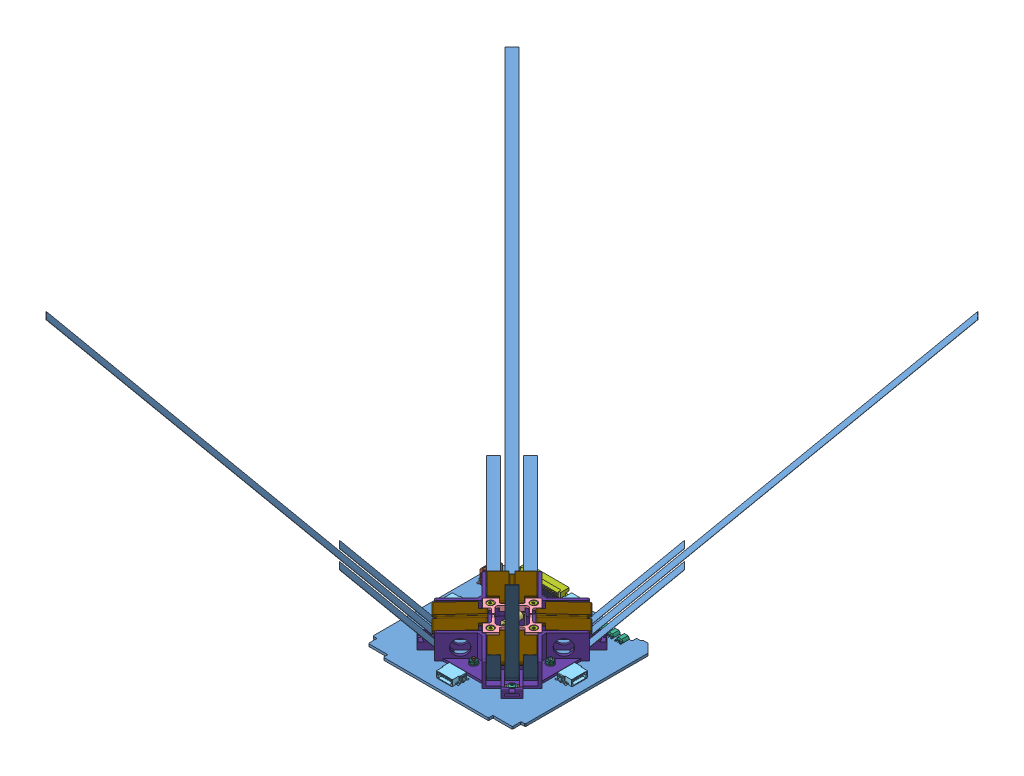
SolidWorks assembly 1U+Zendcard, configuration Deployed. Lengths in mm.
Overall size (309.73 193.28 309.73).
94 component instances, 25 part files, 155 mates.
Components (placement in the parent):
- 1UEndCardPCB-1: 1UEndCardPCB [Circular Turnstile] at origin
- m55-7011242_asm-2: m55-7011242_asm [Default] at (-42.5 0.8 -28.9) x (0 0 1) z (0 1 0) size (12.7 7.2 9)
  - m55-7011242_asm.stp-1: m55-7011242_asm.stp [Default] at origin size (12.7 7.2 9)
    - M55-70112_MOULD.stp-1: M55-70112_MOULD.stp [Default] at origin size (12.7 4.2 9)
    - M55-701_CONTACT.stp-1: M55-701_CONTACT.stp [Default] at (-3.175 -0.785 7.25) x (1 0 0) z (0 1 0) size (1.1 7.25 2.42)
    - M55-701_CONTACT.stp-2: M55-701_CONTACT.stp [Default] at (-1.905 -0.785 7.25) x (1 0 0) z (0 1 0) size (1.1 7.25 2.42)
    - M55-701_CONTACT.stp-3: M55-701_CONTACT.stp [Default] at (-0.635 -0.785 7.25) x (1 0 0) z (0 1 0) size (1.1 7.25 2.42)
    - M55-701_CONTACT.stp-4: M55-701_CONTACT.stp [Default] at (0.635 -0.785 7.25) x (1 0 0) z (0 1 0) size (1.1 7.25 2.42)
    - M55-701_CONTACT.stp-5: M55-701_CONTACT.stp [Default] at (1.905 -0.785 7.25) x (1 0 0) z (0 1 0) size (1.1 7.25 2.42)
    - M55-701_CONTACT.stp-6: M55-701_CONTACT.stp [Default] at (3.175 -0.785 7.25) x (1 0 0) z (0 1 0) size (1.1 7.25 2.42)
    - M55-701_CONTACT.stp-7: M55-701_CONTACT.stp [Default] at (-3.175 0.785 7.25) x (-1 0 0) z (0 -1 0) size (1.1 7.25 2.42)
    - M55-701_CONTACT.stp-8: M55-701_CONTACT.stp [Default] at (-1.905 0.785 7.25) x (-1 0 0) z (0 -1 0) size (1.1 7.25 2.42)
    - M55-701_CONTACT.stp-9: M55-701_CONTACT.stp [Default] at (-0.635 0.785 7.25) x (-1 0 0) z (0 -1 0) size (1.1 7.25 2.42)
    - M55-701_CONTACT.stp-10: M55-701_CONTACT.stp [Default] at (0.635 0.785 7.25) x (-1 0 0) z (0 -1 0) size (1.1 7.25 2.42)
    - M55-701_CONTACT.stp-11: M55-701_CONTACT.stp [Default] at (1.905 0.785 7.25) x (-1 0 0) z (0 -1 0) size (1.1 7.25 2.42)
    - M55-701_CONTACT.stp-12: M55-701_CONTACT.stp [Default] at (3.175 0.785 7.25) x (-1 0 0) z (0 -1 0) size (1.1 7.25 2.42)
    - M55-700_STRAP.stp-1: M55-700_STRAP.stp [Default] at (-5.67 0 0) x (1 0 0) z (0 -1 0) size (1 3.25 7.2)
    - M55-700_STRAP.stp-2: M55-700_STRAP.stp [Default] at (5.67 0 0) x (-1 0 0) z (0 1 0) size (1 3.25 7.2)
- m55-7101242_asm_defeature-1: m55-7101242_asm_defeature [Default] at (0 2.9 -35.35) x (-1 0 0) z (0 0 -1)
- m55-7101242_asm_defeature-2: m55-7101242_asm_defeature [Default] at (-35.35 2.9 0) x (0 0 1) z (-1 0 0)
- m55-7101242_asm_defeature-3: m55-7101242_asm_defeature [Default] at (35.35 2.9 0) x (0 0 -1) z (1 0 0)
- m55-7101242_asm_defeature-4: m55-7101242_asm_defeature [Default] at (0 2.9 35.35)
- Molex, LLC 0733000020 (Card Connector)-1: Molex, LLC 0733000020 (Card Connector) [Default] at (22.001 0.9778 -40.8) x (-1 0 0) z (0 0 -1)
- Molex, LLC 0733000020 (Card Connector)-2: Molex, LLC 0733000020 (Card Connector) [Default] at (28.001 0.9778 -40.8) x (-1 0 0) z (0 0 -1)
- Molex, LLC 0733000020 (Card Connector)-3: Molex, LLC 0733000020 (Card Connector) [Default] at (33.999 0.9778 -40.8) x (-1 0 0) z (0 0 -1)
- TFM_120_01_L_D_RA-1: TFM_120_01_L_D_RA [Default] at (-21.65 3.6575 -39.237) x (-1 0 0) z (0 -1 0) size (28.58 7.49 7.62)
  - _TFM_120_01_L_D_RA_terminal_2-1: _TFM_120_01_L_D_RA_terminal_2 [Default] at origin size (28.58 5.59 5.72)
  - _TFM_120_01_L_D_RA_pins_4-1: _TFM_120_01_L_D_RA_pins_4 [Default] at origin size (25.4 6.95 5.84)
- MezzaninePCB-1: MezzaninePCB [Default] at (0 -4.4 0) x (1 0 0) z (0 1 0)
- R107.064.070C-1: R107.064.070C [Default] at (23.4 -2.8 -23.4) x (0 1 0) z (0.707107 0 -0.707107)
- R107.064.070C-2: R107.064.070C [Default] at (38.1 -2.8 -26.1) x (0 1 0) z (1 0 0)
- R107.064.070C-5: R107.064.070C [Default] at (23.4 -2.8 23.4) x (0 1 0) z (0.707107 0 0.707107)
- R107.064.070C-6: R107.064.070C [Default] at (-23.4 -2.8 23.4) x (0 1 0) z (-0.707107 0 0.707107)
- R107.064.070C-7: R107.064.070C [Default] at (-23.4 -2.8 -23.4) x (0 1 0) z (-0.707107 0 -0.707107)
- 90265A113_18-8 STAINLESS STEEL SHOULDER SCREW-1: 90265A113_18-8 STAINLESS STEEL SHOULDER SCREW [90265A113] at (0 -6.4 -25.1) x (-1 0 0) z (0 -1 0)
- 90265A113_18-8 STAINLESS STEEL SHOULDER SCREW-2: 90265A113_18-8 STAINLESS STEEL SHOULDER SCREW [90265A113] at (0 -6.4 25.1) x (-0.982925 0 0.184007) z (0 -1 0)
- 94669A212_ALUM UNTHRD SPACER-1: 94669A212_ALUM UNTHRD SPACER [94669A212] at (0 -1.8 -25.1) x (-0.837169 0 -0.546944) z (0 1 0)
- 94669A212_ALUM UNTHRD SPACER-2: 94669A212_ALUM UNTHRD SPACER [94669A212] at (0 -1.8 25.1) x (0.982925 0 -0.184007) z (0 1 0)
- 94669A211_ALUM UNTHRD SPACER-3: 94669A211_ALUM UNTHRD SPACER [94669A211] at (25.1 -1.8 0) x (1 0 0) z (0 -1 0)
- 94669A211_ALUM UNTHRD SPACER-4: 94669A211_ALUM UNTHRD SPACER [94669A211] at (-25.1 -1.8 0) x (1 0 0) z (0 -1 0)
- 92855A840_18-8 SS LOW-PROFILE SCKT HEAD SCREWS-1: 92855A840_18-8 SS LOW-PROFILE SCKT HEAD SCREWS [92855A840] at (-25.1 5.6 0) x (1 0 0) z (0 1 0)
- 92855A840_18-8 SS LOW-PROFILE SCKT HEAD SCREWS-2: 92855A840_18-8 SS LOW-PROFILE SCKT HEAD SCREWS [92855A840] at (25.1 5.6 0) x (1 0 0) z (0 1 0)
- 91828A111_TYPE 18-8 STAINLESS STEEL HEX NUT-4: 91828A111_TYPE 18-8 STAINLESS STEEL HEX NUT [91828A111] at (-25.1 3.5 0) x (0.837169 0 0.546944) z (0 -1 0)
- 94100A150_18-8 SS PRESS-FIT NUT FOR SOFT MTL PLASTIC-1: 94100A150_18-8 SS PRESS-FIT NUT FOR SOFT MTL PLASTIC [94100A150] at (27.0307 -2.3 27.0307) x (1 0 0) z (0 -1 0)
- 94100A150_18-8 SS PRESS-FIT NUT FOR SOFT MTL PLASTIC-2: 94100A150_18-8 SS PRESS-FIT NUT FOR SOFT MTL PLASTIC [94100A150] at (-27.0307 -2.3 27.0307) x (0 0 1) z (0 -1 0)
- 94100A150_18-8 SS PRESS-FIT NUT FOR SOFT MTL PLASTIC-3: 94100A150_18-8 SS PRESS-FIT NUT FOR SOFT MTL PLASTIC [94100A150] at (-27.0307 -2.3 -27.0307) x (-1 0 0) z (0 -1 0)
- 94100A150_18-8 SS PRESS-FIT NUT FOR SOFT MTL PLASTIC-4: 94100A150_18-8 SS PRESS-FIT NUT FOR SOFT MTL PLASTIC [94100A150] at (27.0307 -2.3 -27.0307) x (0 0 -1) z (0 -1 0)
- TapeMeasureMount-1: TapeMeasureMount [Vented Fastener melt wire] at (0 0.3 0) size (70.66 21.28 70.66)
- Trapdoor-2: Trapdoor [Default] at (-17.0117 16.4693 17.0117) x (-0.707107 0 -0.707107) z (-0.706844 -0.027263 0.706844) size (23 3.2 26)
- TurnstyleElements-1: TurnstyleElements [L band] at (-12.6549 0.8 29.2719) x (-0.707107 0 0.707107) z (-0.707107 0 -0.707107)
- TurnstyleElements-2: TurnstyleElements [L band] at (-24.6757 0.8 17.2511) x (-0.707107 0 0.707107) z (-0.707107 0 -0.707107)
- TurnstyleElements-3: TurnstyleElements [UHF band] at (-18.6653 0.8 23.2615) x (-0.707107 0 0.707107) z (-0.707107 0 -0.707107)
- squarewasher-1: squarewasher [Default] at (-27.3735 2.65 27.3735) x (0.707107 0 0.707107) z (-0.707107 0 0.707107) size (6.5 0.75 5)
- PAC01_VIS-1: PAC01_VIS [Taller Soldering (1U Endcard)] at (0 12.094 8.75) x (0 0 -1) z (0 1 0) size (18.41 4.29 15.59)
- topCap-1: topCap [Default] at (-11.3137 15.4 -0.1414) x (0.707107 0 0.707107) z (-0.707107 0 0.707107) size (27.5 3.5 27.5)
- TurnstyleElements-13: TurnstyleElements [L band] at (-17.2511 0.8 -24.6757) x (-0.707107 0 -0.707107) z (0.707107 0 -0.707107)
- TurnstyleElements-14: TurnstyleElements [L band] at (24.6757 0.8 -17.2511) x (0.707107 0 -0.707107) z (0.707107 0 0.707107)
- TurnstyleElements-15: TurnstyleElements [L band] at (17.2511 0.8 24.6757) x (0.707107 0 0.707107) z (-0.707107 0 0.707107)
- TurnstyleElements-16: TurnstyleElements [UHF band] at (-23.2615 0.8 -18.6653) x (-0.707107 0 -0.707107) z (0.707107 0 -0.707107)
- TurnstyleElements-17: TurnstyleElements [UHF band] at (18.6653 0.8 -23.2615) x (0.707107 0 -0.707107) z (0.707107 0 0.707107)
- TurnstyleElements-18: TurnstyleElements [UHF band] at (23.2615 0.8 18.6653) x (0.707107 0 0.707107) z (-0.707107 0 0.707107)
- TurnstyleElements-19: TurnstyleElements [L band] at (-29.2719 0.8 -12.6549) x (-0.707107 0 -0.707107) z (0.707107 0 -0.707107)
- TurnstyleElements-20: TurnstyleElements [L band] at (12.6549 0.8 -29.2719) x (0.707107 0 -0.707107) z (0.707107 0 0.707107)
- TurnstyleElements-21: TurnstyleElements [L band] at (29.2719 0.8 12.6549) x (0.707107 0 0.707107) z (-0.707107 0 0.707107)
- squarewasher-5: squarewasher [Default] at (-27.3735 2.65 -27.3735) x (-0.707107 0 0.707107) z (-0.707107 0 -0.707107) size (6.5 0.75 5)
- squarewasher-6: squarewasher [Default] at (27.3735 2.65 -27.3735) x (-0.707107 0 -0.707107) z (0.707107 0 -0.707107) size (6.5 0.75 5)
- squarewasher-7: squarewasher [Default] at (27.3735 2.65 27.3735) x (0.707107 0 -0.707107) z (0.707107 0 0.707107) size (6.5 0.75 5)
- Trapdoor-6: Trapdoor [Default] at (-17.0117 16.4693 -17.0117) x (0.707107 0 -0.707107) z (-0.706844 -0.027263 -0.706844) size (23 3.2 26)
- Trapdoor-7: Trapdoor [Default] at (17.0117 16.4693 -17.0117) x (0.707107 0 0.707107) z (0.706844 -0.027263 -0.706844) size (23 3.2 26)
- Trapdoor-8: Trapdoor [Default] at (17.0117 16.4693 17.0117) x (-0.707107 0 0.707107) z (0.706844 -0.027263 0.706844) size (23 3.2 26)
- 94100A150_18-8 SS PRESS-FIT NUT FOR SOFT MTL PLASTIC-5: 94100A150_18-8 SS PRESS-FIT NUT FOR SOFT MTL PLASTIC [94100A150] at (-27.0307 -2.3 -27.0307) x (-1 0 0) z (0 -1 0)
- 90965A110_TYPE 316 STAINLESS STEEL FLAT WASHER-1: 90965A110_TYPE 316 STAINLESS STEEL FLAT WASHER [90965A110] at (-27.0307 3.4 27.0307) x (0 0 -1) z (0 1 0) size (5 5 0.4)
- 90910A922_LOW-PROFILE BUTTON HEAD TORX MACHINE SCREW-1: 90910A922_LOW-PROFILE BUTTON HEAD TORX MACHINE SCREW [90910A922] at (-27.0307 4.9 27.0307) x (1 0 0) z (0 1 0) size (3.8 3.8 7.25)
- 90910A922_LOW-PROFILE BUTTON HEAD TORX MACHINE SCREW-2: 90910A922_LOW-PROFILE BUTTON HEAD TORX MACHINE SCREW [90910A922] at (-27.0307 4.9 -27.0307) x (0 0 1) z (0 1 0) size (3.8 3.8 7.25)
- 90910A922_LOW-PROFILE BUTTON HEAD TORX MACHINE SCREW-3: 90910A922_LOW-PROFILE BUTTON HEAD TORX MACHINE SCREW [90910A922] at (27.0307 4.9 -27.0307) x (-1 0 0) z (0 1 0) size (3.8 3.8 7.25)
- 90910A922_LOW-PROFILE BUTTON HEAD TORX MACHINE SCREW-4: 90910A922_LOW-PROFILE BUTTON HEAD TORX MACHINE SCREW [90910A922] at (27.0307 4.9 27.0307) x (0 0 -1) z (0 1 0) size (3.8 3.8 7.25)
- 90965A110_TYPE 316 STAINLESS STEEL FLAT WASHER-2: 90965A110_TYPE 316 STAINLESS STEEL FLAT WASHER [90965A110] at (-27.0307 3.4 -27.0307) x (1 0 0) z (0 1 0) size (5 5 0.4)
- 90965A110_TYPE 316 STAINLESS STEEL FLAT WASHER-3: 90965A110_TYPE 316 STAINLESS STEEL FLAT WASHER [90965A110] at (27.0307 3.4 -27.0307) x (0 0 1) z (0 1 0) size (5 5 0.4)
- 90965A110_TYPE 316 STAINLESS STEEL FLAT WASHER-4: 90965A110_TYPE 316 STAINLESS STEEL FLAT WASHER [90965A110] at (27.0307 3.4 27.0307) x (-1 0 0) z (0 1 0) size (5 5 0.4)
- 91828A111_TYPE 18-8 STAINLESS STEEL HEX NUT-5: 91828A111_TYPE 18-8 STAINLESS STEEL HEX NUT [91828A111] at (14.1421 12.5 0) x (0.965926 0 -0.258819) z (0 1 0)
- 91828A111_TYPE 18-8 STAINLESS STEEL HEX NUT-6: 91828A111_TYPE 18-8 STAINLESS STEEL HEX NUT [91828A111] at (-14.1421 12.5 0) x (-0.965926 0 0.258819) z (0 1 0)
- 91828A111_TYPE 18-8 STAINLESS STEEL HEX NUT-7: 91828A111_TYPE 18-8 STAINLESS STEEL HEX NUT [91828A111] at (0 12.5 14.1421) x (0.965926 0 -0.258819) z (0 1 0)
- 91828A111_TYPE 18-8 STAINLESS STEEL HEX NUT-8: 91828A111_TYPE 18-8 STAINLESS STEEL HEX NUT [91828A111] at (0 12.5 -14.1421) x (-0.965926 0 0.258819) z (0 1 0)
- 92703A145_18-8 STAINLESS STEEL TORX FLAT HEAD SCREWS (1)-1: 92703A145_18-8 STAINLESS STEEL TORX FLAT HEAD SCREWS (1) [92703A145] at (14.1421 16.75 -0.1414) x (1 0 0) z (0 1 0) size (3.78 3.78 6.2)
- 92703A145_18-8 STAINLESS STEEL TORX FLAT HEAD SCREWS (1)-2: 92703A145_18-8 STAINLESS STEEL TORX FLAT HEAD SCREWS (1) [92703A145] at (0.1414 16.75 14.1421) x (0 0 1) z (0 1 0) size (3.78 3.78 6.2)
- 92703A145_18-8 STAINLESS STEEL TORX FLAT HEAD SCREWS (1)-3: 92703A145_18-8 STAINLESS STEEL TORX FLAT HEAD SCREWS (1) [92703A145] at (-14.1421 16.75 0.1414) x (-1 0 0) z (0 1 0) size (3.78 3.78 6.2)
- 92703A145_18-8 STAINLESS STEEL TORX FLAT HEAD SCREWS (1)-4: 92703A145_18-8 STAINLESS STEEL TORX FLAT HEAD SCREWS (1) [92703A145] at (-0.1414 16.75 -14.1421) x (0 0 -1) z (0 1 0) size (3.78 3.78 6.2)
- 91828A111_TYPE 18-8 STAINLESS STEEL HEX NUT-9: 91828A111_TYPE 18-8 STAINLESS STEEL HEX NUT [91828A111] at (0 3.5 -25.1) x (-0.546944 0 0.837169) z (0 -1 0)
- 91828A111_TYPE 18-8 STAINLESS STEEL HEX NUT-10: 91828A111_TYPE 18-8 STAINLESS STEEL HEX NUT [91828A111] at (25.1 3.5 0) x (-0.837169 0 -0.546944) z (0 -1 0)
- 91828A111_TYPE 18-8 STAINLESS STEEL HEX NUT-11: 91828A111_TYPE 18-8 STAINLESS STEEL HEX NUT [91828A111] at (0 3.5 25.1) x (0.546944 0 -0.837169) z (0 -1 0)
- 90965A110_TYPE 316 STAINLESS STEEL FLAT WASHER-5: 90965A110_TYPE 316 STAINLESS STEEL FLAT WASHER [90965A110] at (-25.1 2.7 0) x (0.546944 0 -0.837169) z (0 -1 0) size (5 5 0.4)
- 90965A110_TYPE 316 STAINLESS STEEL FLAT WASHER-6: 90965A110_TYPE 316 STAINLESS STEEL FLAT WASHER [90965A110] at (0 2.7 -25.1) x (0.837169 0 0.546944) z (0 -1 0) size (5 5 0.4)
- 90965A110_TYPE 316 STAINLESS STEEL FLAT WASHER-7: 90965A110_TYPE 316 STAINLESS STEEL FLAT WASHER [90965A110] at (25.1 2.7 0) x (-0.546944 0 0.837169) z (0 -1 0) size (5 5 0.4)
- 90965A110_TYPE 316 STAINLESS STEEL FLAT WASHER-8: 90965A110_TYPE 316 STAINLESS STEEL FLAT WASHER [90965A110] at (0 2.7 25.1) x (-0.837169 0 -0.546944) z (0 -1 0) size (5 5 0.4)
Mates (geometry in assembly coordinates):
- Parallel2: parallel aligned: plane of 1UEndCardPCB-1 through (-49.9 -0.8 0) normal (-1 0 0); plane of m55-7011242_asm-2/m55-7011242_asm.stp-1/M55-70112_MOULD.stp-1 through (-44.6 0.8 -34.57) normal (-1 0 0)
- Concentric1: concentric anti-aligned: cylinder of 1UEndCardPCB-1 through (-42.5 -9.2 -34.285) axis (0 1 0) radius 0.8; circle of m55-7011242_asm-2/m55-7011242_asm.stp-1/M55-70112_MOULD.stp-1
- Coincident2: coincident anti-aligned: plane of 1UEndCardPCB-1 through (0 0.8 0) normal (0 1 0); plane of m55-7011242_asm-2/m55-7011242_asm.stp-1/M55-700_STRAP.stp-1 through (-42.5 0.8 -34.57) normal (0 -1 0)
- Concentric2: concentric aligned: circle of m55-7101242_asm_defeature-1; cylinder of 1UEndCardPCB-1 through (5.385 -0.8 -37.75) axis (0 1 0) radius 0.8
- Coincident3: coincident anti-aligned: plane of 1UEndCardPCB-1 through (0 0.8 0) normal (0 1 0); plane of m55-7101242_asm_defeature-1 through (5.67 0.8 -35.35) normal (0 -1 0)
- Parallel3: parallel aligned: plane of 1UEndCardPCB-1 through (0 -0.8 -44.8) normal (0 0 -1); plane of m55-7101242_asm_defeature-1 through (0 2.9 -44.15) normal (0 0 -1)
- Coincident4: coincident anti-aligned: plane of 1UEndCardPCB-1 through (0 0.8 0) normal (0 1 0); plane of m55-7101242_asm_defeature-2 through (-35.35 0.8 -5.67) normal (0 -1 0)
- Concentric4: concentric anti-aligned: circle of m55-7101242_asm_defeature-2; cylinder of 1UEndCardPCB-1 through (-37.75 -0.8 -5.385) axis (0 1 0) radius 0.8
- Parallel4: parallel aligned: plane of 1UEndCardPCB-1 through (-49.9 -0.8 0) normal (-1 0 0); plane of m55-7101242_asm_defeature-2 through (-44.15 2.9 0) normal (-1 0 0)
- Coincident6: coincident anti-aligned: plane of 1UEndCardPCB-1 through (0 0.8 0) normal (0 1 0); plane of m55-7101242_asm_defeature-4 through (-5.67 0.8 35.35) normal (0 -1 0)
- Concentric6: concentric anti-aligned: circle of m55-7101242_asm_defeature-4; cylinder of 1UEndCardPCB-1 through (-5.385 -0.8 37.75) axis (0 1 0) radius 0.8
- Parallel5: parallel aligned: plane of m55-7101242_asm_defeature-4 through (0 2.9 44.15) normal (0 0 1); plane of 1UEndCardPCB-1 through (34.4 -0.801 49.8) normal (0 0 1)
- Concentric7: concentric aligned: circle of m55-7101242_asm_defeature-3; cylinder of 1UEndCardPCB-1 through (37.75 -0.8 5.385) axis (0 1 0) radius 0.8
- Coincident7: coincident anti-aligned: plane of 1UEndCardPCB-1 through (0 0.8 0) normal (0 1 0); plane of m55-7101242_asm_defeature-3 through (35.35 0.8 5.67) normal (0 -1 0)
- Parallel6: parallel aligned: plane of 1UEndCardPCB-1 through (49.9 -0.8 0) normal (1 0 0); plane of m55-7101242_asm_defeature-3 through (44.15 2.9 0) normal (1 0 0)
- Coincident18: coincident anti-aligned: plane of 1UEndCardPCB-1 through (0 0.8 0) normal (0 1 0); plane of TFM_120_01_L_D_RA-1/_TFM_120_01_L_D_RA_terminal_2-1 through (-7.3625 0.8 -44.825) normal (0 -1 0)
- Coincident19: coincident: line of 1UEndCardPCB-1 through (-33.8928 0.8 -37.332) axis (0 0 -1); plane of TFM_120_01_L_D_RA-1/_TFM_120_01_L_D_RA_pins_4-1 through (-33.8928 -1.105 -39.999) normal (-1 0 0)
- Coincident20: coincident: line of 1UEndCardPCB-1 through (-9.4072 0.8 -37.332) axis (-1 0 0); plane of TFM_120_01_L_D_RA-1/_TFM_120_01_L_D_RA_pins_4-1 through (-21.65 3.6575 -37.332) normal (0 0 1)
- Coincident22: coincident anti-aligned: plane of 1UEndCardPCB-1 through (0 0.8 0) normal (0 1 0); plane of Molex, LLC 0733000020 (Card Connector)-3 through (33.999 0.8 -35.1866) normal (0 -1 0)
- Coincident23: coincident aligned: plane of 1UEndCardPCB-1 through (0 -0.8 -40.8) normal (0 0 -1); plane of Molex, LLC 0733000020 (Card Connector)-3 through (33.999 -0.6097 -40.8) normal (0 0 -1)
- Distance4: distance = 0.065 mm anti-aligned: plane of Molex, LLC 0733000020 (Card Connector)-3 through (32.475 0.8 -40.8) normal (-1 0 0); plane of 1UEndCardPCB-1 through (32.41 -0.8 0) normal (1 0 0)
- Coincident24: coincident anti-aligned: plane of 1UEndCardPCB-1 through (0 0.8 0) normal (0 1 0); plane of Molex, LLC 0733000020 (Card Connector)-2 through (28.001 0.8 -35.1866) normal (0 -1 0)
- Distance5: distance = 0.065 mm anti-aligned: plane of 1UEndCardPCB-1 through (29.59 -0.8 0) normal (-1 0 0); plane of Molex, LLC 0733000020 (Card Connector)-2 through (29.525 -0.6097 -40.8) normal (1 0 0)
- Coincident25: coincident aligned: plane of 1UEndCardPCB-1 through (0 -0.8 -40.8) normal (0 0 -1); plane of Molex, LLC 0733000020 (Card Connector)-2 through (28.001 -0.6097 -40.8) normal (0 0 -1)
- Coincident26: coincident anti-aligned: plane of 1UEndCardPCB-1 through (0 0.8 0) normal (0 1 0); plane of Molex, LLC 0733000020 (Card Connector)-1 through (22.001 0.8 -35.1866) normal (0 -1 0)
- Distance6: distance = 0.065 mm anti-aligned: plane of Molex, LLC 0733000020 (Card Connector)-1 through (23.525 -0.6097 -40.8) normal (1 0 0); plane of 1UEndCardPCB-1 through (23.59 -0.8 0) normal (-1 0 0)
- Coincident27: coincident aligned: plane of 1UEndCardPCB-1 through (0 -0.8 -40.8) normal (0 0 -1); plane of Molex, LLC 0733000020 (Card Connector)-1 through (22.001 -0.6097 -40.8) normal (0 0 -1)
- Coincident64: coincident anti-aligned: plane of 1UEndCardPCB-1 through (0 -0.8 0) normal (0 -1 0); plane of tunacan-1 through (5.1664 1.6055 -5.6105) normal (0 1 0)
- Concentric9: concentric aligned: circle of EndCardPCB-1; circle of tunacan-1
- Coincident65: coincident: line of 1UEndCardPCB-1 through (0 0.8 5.2282) axis (0 0 -1); plane of tunacan-1 through (5.1664 -24.6445 -5.6105) normal (1 0 0)
- Coincident70: coincident anti-aligned: plane of 1UEndCardPCB-1 through (0 -0.8 0) normal (0 -1 0); plane of halfinTurnstileMount-12 through (-25.9822 1.6055 27.1766) normal (0 1 0)
- Coincident72: coincident aligned: plane of halfinTurnstileMount-12 through (-25.9822 1.6055 27.1766) normal (0 0 -1); plane of Turnstile_Antenna-4 through (-153.4531 -161.0492 27.1766) normal (0 0 -1)
- Parallel22: parallel aligned: cylinder of halfinTurnstileMount-12 through (-5.5264 -13.1224 27.1766) axis (-0.707107 -0.707107 0) radius 25; cylinder of Turnstile_Antenna-4 through (-11.8904 -19.4864 27.1766) axis (-0.707107 -0.707107 0) radius 25
- Concentric11: concentric aligned: cylinder of halfinTurnstileMount-12 through (-5.5264 -13.1224 27.1766) axis (-0.707107 -0.707107 0) radius 25; cylinder of Turnstile_Antenna-4 through (-11.8904 -19.4864 27.1766) axis (-0.707107 -0.707107 0) radius 25
- Coincident73: coincident anti-aligned: plane of 1UEndCardPCB-1 through (0 -0.8 0) normal (0 -1 0); plane of halfinTurnstileMount-13 through (-27.6207 1.6055 -30.4458) normal (0 1 0)
- Coincident74: coincident anti-aligned: plane of 1UEndCardPCB-1 through (0 -0.8 0) normal (0 -1 0); plane of halfinTurnstileMount-11 through (30.0017 1.6055 -32.0842) normal (0 1 0)
- Coincident80: coincident anti-aligned: plane of Turnstile_Antenna-1 through (15.9098 -19.4864 -32.0842) normal (0 0 -1); plane of halfinTurnstileMount-11 through (30.0017 1.6055 -32.0842) normal (0 0 1)
- Tangent1: tangent aligned: cylinder of Turnstile_Antenna-1 through (157.4726 -161.0492 -32.0842) axis (-0.707107 0.707107 0) radius 25; cylinder of halfinTurnstileMount-11 through (9.5459 -13.1224 -32.0842) axis (0.707107 -0.707107 0) radius 25
- Coincident81: coincident anti-aligned: plane of 1UEndCardPCB-1 through (0 -0.8 0) normal (0 -1 0); plane of halfinTurnstileMount-14 through (31.6402 1.6055 25.5382) normal (0 1 0)
- Coincident82: coincident aligned: plane of halfinTurnstileMount-14 through (31.6402 1.6055 25.5382) normal (-1 0 0); plane of Turnstile_Antenna-3 through (31.6402 -161.0492 153.0091) normal (-1 0 0)
- Tangent2: tangent aligned: cylinder of halfinTurnstileMount-14 through (31.6402 -13.1224 5.0823) axis (0 -0.707107 0.707107) radius 25; cylinder of Turnstile_Antenna-3 through (31.6402 -19.4864 11.4463) axis (0 -0.707107 0.707107) radius 25
- Tangent3: tangent aligned: cylinder of halfinTurnstileMount-13 through (-27.6207 -13.1224 -9.9899) axis (0 -0.707107 -0.707107) radius 25; cylinder of Turnstile_Antenna-2 through (-27.6207 -19.4864 -16.3539) axis (0 -0.707107 -0.707107) radius 25
- Coincident92: coincident anti-aligned: circle of tunacan-1; plane of HARP-9002-A-2/HARP-9002-A.stp-1/navitar-solid-model_swir-25.stp-1 through (5.1664 -50.8945 -14.8605) normal (0 -1 0)
- Concentric12: concentric aligned: circle of tunacan-1; circle of HARP-9002-A-2/HARP-9002-A.stp-1/navitar-solid-model_swir-25.stp-1
- Parallel27: parallel aligned: plane of 1UEndCardPCB-1 through (0 -0.8 49.9) normal (0 0 1); plane of HARP-9002-A-2/HARP-9002-A.stp-1/instrument_electronics.stp-1/TIM PCB.stp-1 through (-41.2572 22.5257 42.352) normal (0 0 1)
- Coincident93: coincident aligned: plane of halfinTurnstileMount-13 through (-27.6207 1.6055 -30.4458) normal (1 0 0); plane of Turnstile_Antenna-2 through (-27.6207 -161.0492 -157.9167) normal (1 0 0)
- Tangent4: tangent aligned: cylinder of halfinTurnstileMount-13 through (-27.6207 -13.1224 -9.9899) axis (0 -0.707107 -0.707107) radius 25; cylinder of Turnstile_Antenna-2 through (-27.6207 -19.4864 -16.3539) axis (0 -0.707107 -0.707107) radius 25
- Parallel28: parallel aligned: cylinder of halfinTurnstileMount-13 through (-27.6207 -13.1224 -9.9899) axis (0 -0.707107 -0.707107) radius 25; cylinder of Turnstile_Antenna-2 through (-27.6207 -19.4864 -16.3539) axis (0 -0.707107 -0.707107) radius 25
- Coincident94: coincident anti-aligned: plane of halfinTurnstileMount-12 through (-29.4822 -1.8945 27.1766) normal (-0.707107 -0.707107 0); plane of Turnstile_Antenna-4 through (-11.8904 -19.4864 27.1766) normal (0.707107 0.707107 0)
- Coincident95: coincident anti-aligned: plane of halfinTurnstileMount-13 through (-27.6207 -1.8945 -33.9458) normal (0 -0.707107 -0.707107); plane of Turnstile_Antenna-2 through (-27.6207 -19.4864 -16.3539) normal (0 0.707107 0.707107)
- Coincident96: coincident anti-aligned: plane of Turnstile_Antenna-1 through (15.9098 -19.4864 -32.0842) normal (-0.707107 0.707107 0); plane of halfinTurnstileMount-11 through (33.5017 -1.8945 -32.0842) normal (0.707107 -0.707107 0)
- Coincident97: coincident anti-aligned: plane of halfinTurnstileMount-14 through (31.6402 -1.8945 29.0382) normal (0 -0.707107 0.707107); plane of Turnstile_Antenna-3 through (31.6402 -19.4864 11.4463) normal (0 0.707107 -0.707107)
- Coincident99: coincident: plane of halfinTurnstileMount-9; point of tunacan-1
- Coincident100: coincident anti-aligned: plane of halfinTurnstileMount-10; plane of halfinTurnstileMount-9
- Coincident101: coincident aligned: line of halfinTurnstileMount-11 through (40.353 -0.3945 -21.7864) axis (0 0 -1); line of halfinTurnstileMount-9 through (43.3496 -0.3945 21.665) axis (0 0 -1)
- Coincident103: coincident anti-aligned: plane of halfinTurnstileMount-6; plane of halfinTurnstileMount-11
- Coincident104: coincident aligned: line of halfinTurnstileMount-6 through (-19.1125 -0.3945 29.5761) axis (1 0 0); line of halfinTurnstileMount-9 through (24.3389 -0.3945 32.5726) axis (1 0 0)
- Coincident106: coincident: line of EndCardPCB-1 through (-30.0202 1.6055 -40.7971) axis (0 0 1); plane of halfinTurnstileMount-10 through (-30.0202 37.1592 -40.7971) normal (-1 0 0)
- Coincident108: coincident: line of EndCardPCB-1 through (-30.0202 1.6055 -40.7971) axis (0 0 1); plane of halfinTurnstileMount-6 through (-30.0202 37.1592 29.5761) normal (-1 0 0)
- Coincident109: coincident: line of EndCardPCB-1 through (-30.0202 1.6055 29.5761) axis (1 0 0); plane of halfinTurnstileMount-6 through (-30.0202 37.1592 29.5761) normal (0 0 1)
- Coincident121: coincident anti-aligned: plane of halfinTurnstileMount-12 through (-17.1447 4.6055 35.8895) normal (0 0 1); line of 1UEndCardPCB-1 through (-41.5 -0.8 41.5) axis (1 0 0)
- Coincident122: coincident: line of 1UEndCardPCB-1 through (-41.5 0.8 46.9) axis (0 0 -1); plane of halfinTurnstileMount-12 through (-36.3336 4.6055 35.8895) normal (-1 0 0)
- Coincident123: coincident: line of 1UEndCardPCB-1 through (-41.5 0.8 46.9) axis (0 0 -1); plane of halfinTurnstileMount-13 through (-36.3336 4.6055 -21.6083) normal (-1 0 0)
- Coincident124: coincident: line of 1UEndCardPCB-1 through (-35.1866 -0.8 -35.1866) axis (1 0 0); plane of halfinTurnstileMount-13 through (-36.3336 4.6055 -40.7971) normal (0 0 -1)
- Coincident125: coincident: line of 1UEndCardPCB-1 through (-35.1866 -0.8 -35.1866) axis (1 0 0); plane of halfinTurnstileMount-11 through (21.1642 4.6055 -40.7971) normal (0 0 -1)
- Coincident126: coincident: line of 1UEndCardPCB-1 through (35.1866 -0.8 -35.1866) axis (0 0 1); plane of halfinTurnstileMount-11 through (40.353 4.6055 -40.7971) normal (1 0 0)
- Coincident127: coincident aligned: line of 1UEndCardPCB-1 through (-41.5 -0.8 41.5) axis (1 0 0); plane of halfinTurnstileMount-14 through (40.353 4.6055 35.8895) normal (0 0 1)
- Coincident128: coincident: line of 1UEndCardPCB-1 through (35.1866 -0.8 -35.1866) axis (0 0 1); plane of halfinTurnstileMount-14 through (40.353 4.6055 16.7007) normal (1 0 0)
- Coincident129: coincident anti-aligned: plane of 1UEndCardPCB-1 through (0 -0.8 0) normal (0 -1 0); plane of Turnstile Mount-1 through (32.503 1.6055 18.8895) normal (0 1 0)
- Coincident130: coincident aligned: line of 1UEndCardPCB-1 through (35.1866 -0.8 -35.1866) axis (0 0 1); line of Turnstile Mount-1 through (40.353 1.6055 3.8895) axis (0 0 1)
- Coincident131: coincident anti-aligned: line of 1UEndCardPCB-1 through (-41.5 -0.8 41.5) axis (1 0 0); line of Turnstile Mount-1 through (38.353 1.6055 35.8895) axis (-1 0 0)
- Coincident135: coincident anti-aligned: plane of 1UEndCardPCB-1 through (0 -0.8 0) normal (0 -1 0); plane of Turnstile Mount-3 through (23.353 1.6055 -32.9471) normal (0 1 0)
- Coincident136: coincident anti-aligned: plane of 1UEndCardPCB-1 through (0 0.8 0) normal (0 1 0); plane of Turnstile Mount-2 through (11.85 0.8 -16) normal (0 -1 0)
- Coincident142: coincident aligned: line of 1UEndCardPCB-1 through (-35.1866 -0.8 -35.1866) axis (1 0 0); line of Turnstile Mount-3 through (8.353 1.6055 -40.7971) axis (1 0 0)
- Coincident143: coincident aligned: line of 1UEndCardPCB-1 through (35.1866 -0.8 -35.1866) axis (0 0 1); line of Turnstile Mount-3 through (40.353 1.6055 -38.7971) axis (0 0 1)
- Coincident147: coincident aligned: plane of Turnstile Mount-2 through (11.85 0.8 -16) normal (-1 0 0); plane of Turnstile_Antenna-6 through (-27.3366 156.3786 -158.4899) normal (-1 0 0)
- Coincident148: coincident aligned: circle of Turnstile Mount-2; circle of Turnstile_Antenna-6
- Coincident149: coincident anti-aligned: plane of Turnstile Mount-3 through (23.353 1.6055 -32.9471) normal (0 0 1); plane of Turnstile_Antenna-7 through (20.9482 -12.4103 -32.9471) normal (0 0 -1)
- Coincident150: coincident anti-aligned: circle of Turnstile Mount-3; circle of Turnstile_Antenna-7
- Coincident153: coordinate: unknown of EndCardPCB-1
- Coincident154: coincident anti-aligned: plane of Turnstile Mount-2 through (11.85 14.8158 -12.5951) normal (0 0.707107 -0.707107); plane of Rolled Antenna-1 through (11.85 14.8158 -12.5951) normal (0 -0.707107 0.707107)
- Concentric13: concentric anti-aligned: cylinder of Turnstile Mount-2 through (11.85 10.3964 -8.1757) axis (0 0.707107 -0.707107) radius 19.45; cylinder of Rolled Antenna-1 through (11.85 17.4674 -15.2468) axis (0 -0.707107 0.707107) radius 19.45
- Coincident155: coincident aligned: plane of Turnstile Mount-2 through (11.85 0.8 -16) normal (-1 0 0); plane of Rolled Antenna-1 through (11.85 1.0626 -26.3483) normal (-1 0 0)
- Coincident162: coincident: line of 1UEndCardPCB-1 through (75.5 37.75 -0.8) axis (0 -1 0); plane of Turnstile Mount-2 through (27.85 2.3 0) normal (0 0 1)
- Distance7: distance = 4 mm: plane of Turnstile Mount-2 through (4 0.8 -32) normal (-1 0 0); line of 1UEndCardPCB-1 through (0 0.8 5.2282) axis (0 0 -1)
- Coincident163: coincident anti-aligned: plane of 1UEndCardPCB-1 through (0 0.8 0) normal (0 1 0); plane of SFM_120_01_S_D_LC-1/_SFM_120_01_L_D_LC_terminal_2-1 through (-8.95 0.8 -30.046) normal (0 -1 0)
- Coincident164: coincident anti-aligned: plane of TFM_120_01_L_D_RA-1 through (-21.65 3.6575 -39.237) normal (-1 0 0); plane of SFM_120_01_S_D_LC-1 through (-21.65 0.419 -33.094) normal (1 0 0)
- Distance8: distance = 5 mm anti-aligned: unknown of TFM_120_01_L_D_RA-1/_TFM_120_01_L_D_RA_terminal_2-1; plane of SFM_120_01_S_D_LC-1 through (-21.65 0.419 -33.094) normal (0 0 1)
- Distance10: distance = 2 mm anti-aligned: plane of MezzaninePCB-1 through (-26.9 -2.8 -21.1) normal (0 1 0); plane of 1UEndCardPCB-1 through (0 -0.8 0) normal (0 -1 0)
- Coincident169: coincident anti-aligned: plane of MezzaninePCB-1 through (0 -4.4 0) normal (0 0 -1)
- Coincident170: coincident aligned: plane of MezzaninePCB-1 through (0 -4.4 0) normal (1 0 0)
- Coincident171: coincident aligned: plane of MezzaninePCB-1 through (-26.9 -2.8 -21.1) normal (0 1 0); plane of R107.064.070C-1 through (23.4 -2.8 -23.4) normal (0 1 0)
- Coincident176: coincident: line of MezzaninePCB-1 through (24.5314 -2.8 -22.2686) axis (-0.707107 0 -0.707107); plane of R107.064.070C-1 through (23.4 -2.8 -23.4) normal (0.707107 0 -0.707107)
- Coincident177: coincident: line of MezzaninePCB-1 through (0 -2.8 0) axis (0.707107 0 -0.707107); plane of R107.064.070C-1 through (23.4 -2.8 -23.4) normal (0.707107 0 0.707107)
- Coincident178: coincident aligned: plane of MezzaninePCB-1 through (-26.9 -2.8 -21.1) normal (0 1 0); plane of R107.064.070C-2 through (38.1 -2.8 -26.1) normal (0 1 0)
- Coincident180: coincident: line of MezzaninePCB-1 through (38.1 -2.8 -27.7) axis (0 0 1); plane of R107.064.070C-2 through (38.1 -2.8 -26.1) normal (1 0 0)
- Coincident181: coincident: plane of assembly; point of MezzaninePCB-1; plane of R107.064.070C-2 through (38.1 -2.8 -26.1) normal (0 0 1)
- Coincident184: coincident anti-aligned: plane of 1UEndCardPCB-1 through (0 -0.8 0) normal (0 -1 0); plane of 94669A212_ALUM UNTHRD SPACER-2 through (0 -0.8 25.1) normal (0 1 0)
- Concentric16: concentric anti-aligned: cylinder of 90265A113_18-8 STAINLESS STEEL SHOULDER SCREW-2 through (0 5.6 25.1) axis (0 1 0) radius 1.5; cylinder of 94669A212_ALUM UNTHRD SPACER-2 through (0 -0.8 25.1) axis (0 -1 0) radius 2.25
- Coincident185: coincident anti-aligned: plane of 1UEndCardPCB-1 through (0 -0.8 0) normal (0 -1 0); plane of 94669A212_ALUM UNTHRD SPACER-1 through (0 -0.8 -25.1) normal (0 1 0)
- Concentric17: concentric anti-aligned: cylinder of 90265A113_18-8 STAINLESS STEEL SHOULDER SCREW-1 through (0 5.6 -25.1) axis (0 1 0) radius 1.5; cylinder of 94669A212_ALUM UNTHRD SPACER-1 through (0 -0.8 -25.1) axis (0 -1 0) radius 2.25
- Coincident187: coincident anti-aligned: plane of 1UEndCardPCB-1 through (0 -0.8 0) normal (0 -1 0); plane of 94669A211_ALUM UNTHRD SPACER-4 through (-25.1 -0.8 0) normal (0 1 0)
- Coincident188: coincident anti-aligned: plane of 1UEndCardPCB-1 through (0 -0.8 0) normal (0 -1 0); plane of 94669A211_ALUM UNTHRD SPACER-3 through (25.1 -0.8 0) normal (0 1 0)
- Concentric18: concentric aligned: cylinder of 94669A211_ALUM UNTHRD SPACER-3 through (25.1 -2.8 0) axis (0 1 0) radius 2.25; cylinder of 1UEndCardPCB-1 through (25.1 -0.801 0) axis (0 1 0) radius 1.2
- Concentric19: concentric aligned: cylinder of 94669A211_ALUM UNTHRD SPACER-4 through (-25.1 -2.8 0) axis (0 1 0) radius 2.25; cylinder of 1UEndCardPCB-1 through (-25.1 -0.801 0) axis (0 1 0) radius 1.2
- Coincident189: coincident anti-aligned: plane of MezzaninePCB-1 through (-26.9 -4.4 -21.1) normal (0 -1 0); plane of 90265A113_18-8 STAINLESS STEEL SHOULDER SCREW-1 through (0 -4.4 -22.6) normal (0 1 0)
- Coincident190: coincident anti-aligned: plane of MezzaninePCB-1 through (-26.9 -4.4 -21.1) normal (0 -1 0); plane of 90265A113_18-8 STAINLESS STEEL SHOULDER SCREW-2 through (0.46 -4.4 27.5573) normal (0 1 0)
- Coincident191: coincident anti-aligned: plane of MezzaninePCB-1 through (-26.9 -4.4 -21.1) normal (0 -1 0); plane of 92855A840_18-8 SS LOW-PROFILE SCKT HEAD SCREWS-1 through (-25.1 -4.4 0) normal (0 1 0)
- Concentric20: concentric aligned: cylinder of 92855A840_18-8 SS LOW-PROFILE SCKT HEAD SCREWS-1 through (-25.1 -5.75 0) axis (0 1 0) radius 1.9; cylinder of 1UEndCardPCB-1 through (-25.1 -0.801 0) axis (0 1 0) radius 1.2
- Coincident192: coincident anti-aligned: plane of MezzaninePCB-1 through (-26.9 -4.4 -21.1) normal (0 -1 0); plane of 92855A840_18-8 SS LOW-PROFILE SCKT HEAD SCREWS-2 through (25.1 -4.4 0) normal (0 1 0)
- Concentric21: concentric aligned: cylinder of 92855A840_18-8 SS LOW-PROFILE SCKT HEAD SCREWS-2 through (25.1 -5.75 0) axis (0 1 0) radius 1.9; circle of MezzaninePCB-1
- Concentric27: concentric aligned: circle of 92855A840_18-8 SS LOW-PROFILE SCKT HEAD SCREWS-1; circle of 91828A111_TYPE 18-8 STAINLESS STEEL HEX NUT-4
- Coincident201: coincident anti-aligned: plane of 1UEndCardPCB-1 through (0 -0.8 0) normal (0 -1 0); plane of 94100A150_18-8 SS PRESS-FIT NUT FOR SOFT MTL PLASTIC-1 through (27.0307 -0.8 27.0307) normal (0 1 0)
- Concentric30: concentric aligned: cylinder of 1UEndCardPCB-1 through (27.0307 -0.801 27.0307) axis (0 1 0) radius 1.85; circle of 94100A150_18-8 SS PRESS-FIT NUT FOR SOFT MTL PLASTIC-1
- Coincident203: coincident anti-aligned: circle of 1UEndCardPCB-1; circle of TapeMeasureMount-1
- Coincident204: coincident anti-aligned: circle of 1UEndCardPCB-1; circle of TapeMeasureMount-1
- Coincident221: coincident anti-aligned: plane of TapeMeasureMount-1 through (-1.2678 -38.9548 -15.7028) normal (-0.5 -0.707107 0.5); plane of TurnstyleElements-2 through (-32.2019 5.0426 15.5849) normal (0.5 0.707107 -0.5)
- Coincident222: coincident anti-aligned: plane of 1UEndCardPCB-1 through (0 0.8 0) normal (0 1 0); plane of TurnstyleElements-2 through (-29.3419 0.8 12.7249) normal (0 -1 0)
- Coincident223: coincident anti-aligned: plane of TapeMeasureMount-1 through (4.7426 -38.9548 -9.6924) normal (-0.5 -0.707107 0.5); plane of TurnstyleElements-3 through (-26.1915 5.0426 21.5953) normal (0.5 0.707107 -0.5)
- Coincident224: coincident anti-aligned: plane of 1UEndCardPCB-1 through (0 0.8 0) normal (0 1 0); plane of TurnstyleElements-3 through (-23.3315 0.8 18.7353) normal (0 -1 0)
- Coincident225: coincident anti-aligned: plane of TapeMeasureMount-1 through (15.7028 -38.9548 1.2678) normal (-0.5 -0.707107 0.5); plane of TurnstyleElements-1 through (-20.1811 5.0426 27.6057) normal (0.5 0.707107 -0.5)
- Coincident226: coincident anti-aligned: plane of 1UEndCardPCB-1 through (0 0.8 0) normal (0 1 0); plane of TurnstyleElements-1 through (-17.3211 0.8 24.7457) normal (0 -1 0)
- Distance11: distance = 0.25 mm anti-aligned: plane of TurnstyleElements-2 through (-29.2719 0.8 12.6549) normal (-0.707107 0 -0.707107); plane of TapeMeasureMount-1 through (-31.0858 16.8 14.1152) normal (0.707107 0 0.707107)
- Distance12: distance = 0.25 mm anti-aligned: plane of TurnstyleElements-3 through (-23.2615 0.8 18.6653) normal (-0.707107 0 -0.707107); plane of TapeMeasureMount-1 through (21.5398 38.2619 -26.4896) normal (0.707107 0 0.707107)
- Distance13: distance = 0.25 mm anti-aligned: plane of TurnstyleElements-1 through (-17.2511 0.8 24.6757) normal (-0.707107 0 -0.707107); plane of TapeMeasureMount-1 through (-20.4792 38.2619 27.5503) normal (0.707107 0 0.707107)
- Distance14: distance = 0.35 mm anti-aligned: plane of squarewasher-1 through (-27.3735 2.65 27.3735) normal (0 -1 0); plane of TapeMeasureMount-1 through (0 2.3 0) normal (0 1 0)
- Parallel31: parallel: line of TapeMeasureMount-1 through (-22.9541 2.3 27.9038) axis (-0.707107 0 -0.707107); plane of squarewasher-1 through (-27.9038 3.4 23.3076) normal (0.707107 0 -0.707107)
- Parallel32: parallel: line of TapeMeasureMount-1 through (-28.6109 2.3 33.5607) axis (0.707107 0 -0.707107); plane of squarewasher-1 through (-26.8431 3.4 31.4393) normal (0.707107 0 0.707107)
- Concentric38: concentric aligned: circle of TapeMeasureMount-1; circle of squarewasher-1
- Coincident243: coincident anti-aligned: plane of PAC01_VIS-1 through (0 12.094 8.75) normal (-1 0 0)
- Coincident248: coincident anti-aligned: plane of 1UEndCardPCB-1 through (0 0.8 0) normal (0 1 0); plane of PAC01_VIS-1 through (0 0.8 -8.751) normal (0 -1 0)
- Coincident247: coincident: line of PAC01_VIS-1 through (0 16.3863 0) axis (0 -1 0)
- Concentric42: concentric aligned: circle of TapeMeasureMount-1; circle of Trapdoor-2
- Distance17: distance = 6 mm aligned: plane of Trapdoor-2 through (-17.0117 16.4693 17.0117) normal (-0.707107 0 -0.707107); plane of TapeMeasureMount-1 through (-5.6569 13.3 14.1421) normal (-0.707107 0 -0.707107)
- Distance19: distance = 0.15 mm anti-aligned: plane of TapeMeasureMount-1 through (-5.6569 15.4 -14.1421) normal (0.707107 0 0.707107); plane of topCap-1 through (-19.4454 13.3 -0.1414) normal (-0.707107 0 -0.707107)
- Distance18: distance = 0.15 mm anti-aligned: plane of TapeMeasureMount-1 through (5.6569 15.4 -14.1421) normal (-0.707107 0 0.707107); plane of topCap-1 through (0 13.3 -19.5869) normal (0.707107 0 -0.707107)
- Coincident260: coincident anti-aligned: plane of TapeMeasureMount-1 through (0 15.4 0) normal (0 1 0); plane of topCap-1 through (0 15.4 -11.4551) normal (0 -1 0)
- Coincident261: coincident aligned: circle of squarewasher-1; circle of 90965A110_TYPE 316 STAINLESS STEEL FLAT WASHER-1
- Coincident263: coincident anti-aligned: plane of 90965A110_TYPE 316 STAINLESS STEEL FLAT WASHER-1 through (-27.0307 3.8 27.0307) normal (0 1 0); plane of 90910A922_LOW-PROFILE BUTTON HEAD TORX MACHINE SCREW-1 through (-27.0307 3.8 28.9307) normal (0 -1 0)
- Concentric48: concentric aligned: circle of 90965A110_TYPE 316 STAINLESS STEEL FLAT WASHER-1; circle of 90910A922_LOW-PROFILE BUTTON HEAD TORX MACHINE SCREW-1
- Parallel34: parallel anti-aligned: plane of 90910A922_LOW-PROFILE BUTTON HEAD TORX MACHINE SCREW-1 through (-27.0307 4.9 27.0307) normal (0 0 -1)
- Parallel35: parallel anti-aligned: plane of 90965A110_TYPE 316 STAINLESS STEEL FLAT WASHER-1 through (-27.0307 3.4 27.0307) normal (0 0 -1)
- Coincident269: coincident anti-aligned: plane of TapeMeasureMount-1 through (0 13.3 0) normal (0 -1 0); plane of 91828A111_TYPE 18-8 STAINLESS STEEL HEX NUT-5 through (11.9114 13.3 -0.5977) normal (0 1 0)
- Concentric49: concentric anti-aligned: circle of TapeMeasureMount-1; circle of 91828A111_TYPE 18-8 STAINLESS STEEL HEX NUT-5
- Parallel36: parallel anti-aligned: plane of TapeMeasureMount-1 through (12.3744 13.3 1.7678) normal (0.965926 0 -0.258819); plane of 91828A111_TYPE 18-8 STAINLESS STEEL HEX NUT-5 through (11.9114 13.3 -0.5977) normal (-0.965926 0 0.258819)
- Coincident271: coincident anti-aligned: plane of TapeMeasureMount-1 through (0 13.3 0) normal (0 -1 0); plane of 91828A111_TYPE 18-8 STAINLESS STEEL HEX NUT-7 through (-2.2307 13.3 13.5444) normal (0 1 0)
- Concentric50: concentric anti-aligned: circle of TapeMeasureMount-1; circle of 91828A111_TYPE 18-8 STAINLESS STEEL HEX NUT-7
- Parallel37: parallel anti-aligned: plane of TapeMeasureMount-1 through (-1.7678 13.3 15.9099) normal (0.965926 0 -0.258819); plane of 91828A111_TYPE 18-8 STAINLESS STEEL HEX NUT-7 through (-2.2307 13.3 13.5444) normal (-0.965926 0 0.258819)
- Coincident273: coincident aligned: cone of topCap-1 through (14.1421 16.8 -0.1414) axis (0 -1 0); cone of 92703A145_18-8 STAINLESS STEEL TORX FLAT HEAD SCREWS (1)-1 through (14.1421 15.55 -0.1414) axis (0 -1 0)
- Coincident274: coincident anti-aligned: plane of TapeMeasureMount-1 through (0 2.3 0) normal (0 1 0); plane of 90965A110_TYPE 316 STAINLESS STEEL FLAT WASHER-5 through (-25.1 2.3 0) normal (0 -1 0)
- Concentric52: concentric anti-aligned: circle of TapeMeasureMount-1; circle of 90965A110_TYPE 316 STAINLESS STEEL FLAT WASHER-5
- Coincident275: coincident anti-aligned: plane of 91828A111_TYPE 18-8 STAINLESS STEEL HEX NUT-4 through (-27.4059 2.7 -0.1272) normal (0 -1 0); plane of 90965A110_TYPE 316 STAINLESS STEEL FLAT WASHER-5 through (-25.1 2.7 0) normal (0 1 0)
- Concentric53: concentric anti-aligned: circle of 90265A113_18-8 STAINLESS STEEL SHOULDER SCREW-2; circle of 90965A110_TYPE 316 STAINLESS STEEL FLAT WASHER-8
- Parallel38: parallel anti-aligned: plane of TapeMeasureMount-1 through (0 14.35 0) normal (0 1 0); plane of Trapdoor-2 through (-2.4798 14.7154 18.7433) normal (0 -1 0)
- Concentric54: concentric aligned: circle of MezzaninePCB-1; circle of 94669A212_ALUM UNTHRD SPACER-1
